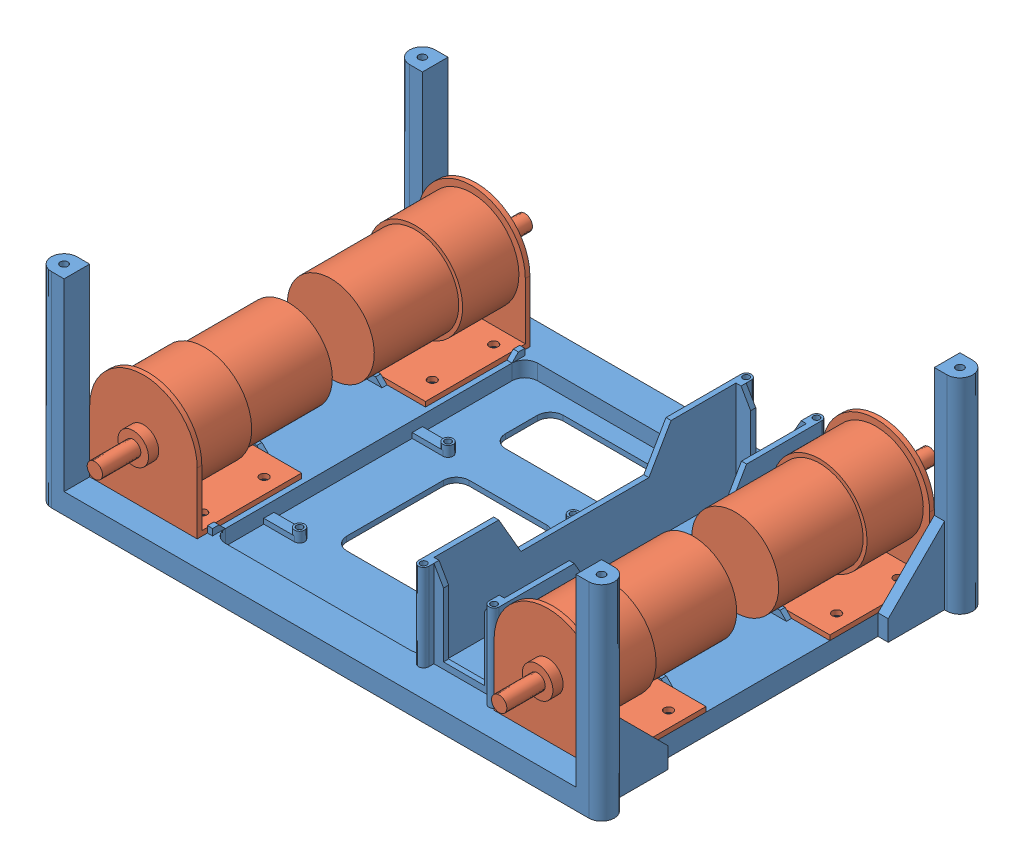
SolidWorks assembly 装配体1, configuration Default. Lengths in mm.
Overall size (220 80 168).
5 component instances, 2 part files, 12 mates.
Components (placement in the parent):
- 底盘-1: 底盘 [默认] at origin size (220 80 150)
- 电机-1: 电机 [默认] at (79 32 41.2) x (1 0 0) z (0 1 0) size (42 75.8 45)
- 电机-2: 电机 [默认] at (79 32 -41.2) x (-1 0 0) z (0 1 0) size (42 75.8 45)
- 电机-3: 电机 [默认] at (-79 32 41.2) x (1 0 0) z (0 1 0) size (42 75.8 45)
- 电机-4: 电机 [默认] at (-79 32 -41.2) x (-1 0 0) z (0 1 0) size (42 75.8 45)
Mates (geometry in assembly coordinates):
- 同心1: concentric: circle of 底盘-1; circle of 电机-1
- 同心2: concentric: circle of 底盘-1; circle of 电机-1
- 重合1: coincident anti-aligned: plane of 底盘-1 through (0 8 0) normal (0 1 0); plane of 电机-1 through (100 8 65) normal (0 -1 0)
- 同心3: concentric: circle of 底盘-1; circle of 电机-2
- 同心4: concentric: circle of 底盘-1; circle of 电机-2
- 重合2: coincident anti-aligned: plane of 底盘-1 through (0 8 0) normal (0 1 0); plane of 电机-2 through (58 8 -65) normal (0 -1 0)
- 同心5: concentric: circle of 底盘-1; circle of 电机-3
- 同心6: concentric: circle of 底盘-1; circle of 电机-3
- 重合3: coincident anti-aligned: plane of 底盘-1 through (0 8 0) normal (0 1 0); plane of 电机-3 through (-58 8 65) normal (0 -1 0)
- 同心7: concentric: circle of 底盘-1; circle of 电机-4
- 同心8: concentric: circle of 底盘-1; circle of 电机-4
- 重合4: coincident anti-aligned: plane of 底盘-1 through (0 8 0) normal (0 1 0); plane of 电机-4 through (-100 8 -65) normal (0 -1 0)
